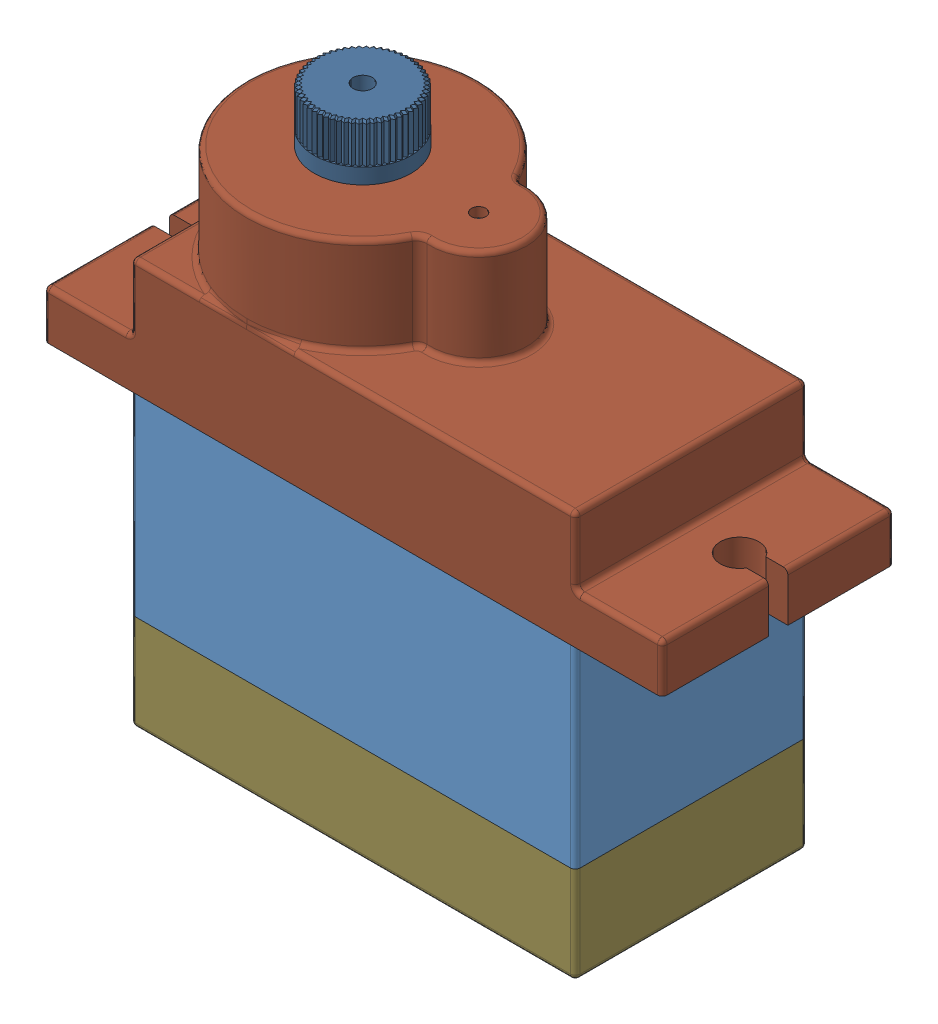
SolidWorks assembly SERVO 2, configuration Default. Lengths in mm.
Overall size (32 28.96 14.19).
25 component instances, 14 part files, 47 mates.
Components (placement in the parent):
- middle cover-1: middle cover [Default] at (8.87 8.8972 15.8774) size (23 11 12)
- shaft-1: shaft [Default] at (3.37 15.3972 15.8774) x (0 1 0) z (-0.985923 0 -0.167197) size (14.5 8.25 8.81)
- part 1-1: part 1 [Default] at (3.37 15.7972 15.8774) x (0 0 1) z (1 0 0) size (9.5 5.14 9.55)
- gear_sub1-1: gear_sub1 [Default] at (9.5 19.3472 15.8774) x (-0.853456 0 0.521165) z (-0.521165 0 -0.853456) size (10.24 10.65 10.25)
  - shaft^gear_sub1-1: shaft^gear_sub1 [Default] at origin size (1 10.65 1) (virtual)
  - spur gear_iso-2: spur gear_iso [ISO - Spur gear 0.25M 39T 20PA 1FW ---S39A75H50L0.8N] at (0 0.1 0) x (0 1 0) z (0 0 1) size (1 10.24 10.25)
  - spur gear_iso-5: spur gear_iso [ISO - Spur gear 0.25M 10T 20PA 1.75FW ---S10A75H50L1.0N] at (0 1.1 0) x (0 1 0) z (0 0 1) size (1.75 2.87 3)
- gear_sub2-1: gear_sub2 [Default] at (3.37 20.7972 15.8774) x (-0.834296 0 0.551317) z (-0.551317 0 -0.834296) size (10.24 2.75 10.25)
  - spur gear_iso-2: spur gear_iso [ISO - Spur gear 0.25M 39T 20PA 1FW ---S39A75H50L0.8N] at (0 0.1 0) x (0 1 0) z (0 0 1) size (1 10.24 10.25)
  - spur gear_iso-5: spur gear_iso [ISO - Spur gear 0.25M 10T 20PA 1.75FW ---S10A75H50L1.0N] at (0 1.1 0) x (0 1 0) z (0 0 1) size (1.75 2.87 3)
- pcb-1: pcb [Default] at (4.7516 11.69 15.8774) x (0.906308 0.422618 0) z (0 0 -1) size (10 2 9)
- wires1^SERVO 2-1: wires1^SERVO 2 [Default] at (8.87 8.8972 21.8774) (virtual)
- DC Motor as part-2: DC Motor as part [Default] at (20.0465 3.7393 19.3612) x (0 0 -1) z (0 1 0) size (8.04 6.55 11.14)
- Rotor scaled-1: Rotor scaled [Default] at (15.62 14.0372 15.8774) x (0.826635 0 -0.562739) z (0 1 0) size (5.2 5.12 15.2)
- spur gear_am-3: spur gear_am [Metric - Spur gear 0.25M 10T 20PA 2FW ---S10N75H50L0.8N] at (15.62 18.9472 15.8774) x (0 1 0) z (0.067436 0 0.997724) size (2 2.87 3)
- gear_sub3-2: gear_sub3 [Default] at (9.5126 21.8914 14.1824) x (-0.43734 0 -0.899296) z (0.899296 0 -0.43734) size (10.24 7 10.25)
  - spur gear_iso-2: spur gear_iso [ISO - Spur gear 0.25M 39T 20PA 1FW ---S39A75H50L0.8N] at (-1.5188 0.3058 -0.7526) x (0 1 0) z (0 0 1) size (1 10.24 10.25)
  - spur gear_iso-6: spur gear_iso [ISO - Spur gear 0.25M 10T 20PA 6FW ---S10A75H50L0.8N] at (-1.5188 1.3058 -0.7526) x (0 1 0) z (0 0 1) size (6 2.87 3)
- gear5-1: gear5 [Default] at (0.4816 -19.0533 15.951) x (0 -1 0) z (0.847043 0 0.531525) size (6.5 10.24 10.25)
- Part5-1: Part5 [Default] at (8.87 24.8972 15.8774) size (32 11 12.1)
- part 3 bottom-1: part 3 bottom [Default] at (8.87 3.8972 15.8774) size (23 5 12)
- Part6-1: Part6 [Default] at (-1.38 3.7472 11.1274) x (0 1 0) z (-0.44899 0 0.893537) size (20.01 2 2)
- Part6-2: Part6 [Default] at (-1.38 3.7472 20.6274) x (0 1 0) z (-0.272553 0 0.962141) size (20.01 2 2)
- Part6-4: Part6 [Default] at (19.12 3.7472 20.6274) x (0 1 0) z (-0.058733 0 0.998274) size (20.01 2 2)
- Part6-6: Part6 [Default] at (19.12 3.7472 11.1274) x (0 1 0) z (0.17693 0 0.984223) size (20.01 2 2)
Mates (geometry in assembly coordinates):
- Concentric1: concentric anti-aligned: cylinder of middle cover-1 through (3.37 8.8962 15.8774) axis (0 1 0) radius 5; cylinder of part 1-1 through (3.37 16.2972 15.8774) axis (0 -1 0) radius 4.75
- Concentric2: concentric aligned: cylinder of shaft-1 through (3.37 15.3972 15.8774) axis (0 -1 0) radius 0.6; cylinder of part 1-1 through (3.37 19.2972 15.8774) axis (0 -1 0) radius 4.5
- Tangent1: tangent: face of shaft-1; plane of part 1-1 through (4.8064 16.4472 14.6722) normal (0 1 0)
- Concentric3: concentric aligned: cylinder of shaft-1 through (3.37 15.3972 15.8774) axis (0 -1 0) radius 0.5; cylinder of gear_sub2-1/spur gear_iso-5 through (3.37 71.8973 15.8774) axis (0 -1 0) radius 0.5
- Coincident6: coincident anti-aligned: plane of shaft-1 through (3.4536 20.8972 15.3844) normal (0 1 0); plane of gear_sub2-1/spur gear_iso-2 through (3.37 20.8972 15.8774) normal (0 -1 0)
- Concentric4: concentric aligned: cylinder of middle cover-1 through (9.5 19.4472 15.8774) axis (0 -1 0) radius 0.5; cylinder of gear_sub1-1/shaft^gear_sub1-1 through (9.5 18.6972 15.8774) axis (0 -1 0) radius 0.5
- Width1: width anti-aligned: plane of pcb-1 through (9.6001 13.1234 20.3774) normal (0 0 1); plane of pcb-1 through (9.6001 13.1234 11.3774) normal (0 0 -1); plane of middle cover-1 through (20.37 18.8972 20.8774) normal (0 0 -1); plane of middle cover-1 through (20.37 18.8972 10.8774) normal (0 0 1)
- Coincident9: coincident: plane of middle cover-1 through (8.87 8.8972 15.8774) normal (0 -1 0); line of pcb-1 through (0.537 8.8972 20.3774) axis (0 0 -1)
- Angle1: planar angle = 0.436332 rad aligned: plane of pcb-1 through (5.0685 11.0103 15.8774) normal (0.422618 -0.906308 0); plane of middle cover-1 through (8.87 8.8972 15.8774) normal (0 -1 0)
- Tangent2: tangent: cylinder of middle cover-1 through (-1.38 18.8972 20.6274) axis (0 -1 0) radius 1.6; line of pcb-1 through (0.22 9.5769 20.3774) axis (0 0 -1)
- InPlace1: in place: plane of middle cover-1 through (20.37 18.8972 21.8774) normal (0 0 1); plane of ? through (0 0 21.8774) normal (0 0 1); moOrthogonalPlaneRef_w of middle cover-1 through (20.37 18.8972 21.8774) normal (0 0 1); plane of ? through (0 0 21.8774) normal (0 1 0); plane of middle cover-1 through (20.37 18.8972 21.8774) normal (0 0 1); plane of ? through (0 0 21.8774) normal (1 0 0); plane of middle cover-1 through (20.37 18.8972 21.8774) normal (0 0 1); unknown of wires1^SERVO 2-1
- Coincident11: coincident aligned: plane of middle cover-1; plane of wires1^SERVO 2-1
- Coincident12: coincident aligned: moOrthogonalPlaneRef_w of middle cover-1 through (8.87 8.8972 21.8774) normal (0 1 0); plane of wires1^SERVO 2-1 through (8.87 8.8972 21.8774) normal (0 1 0)
- Coincident13: coincident anti-aligned: moOrthogonalPlaneRef_w of middle cover-1 through (8.87 8.8972 21.8774) normal (-1 0 0); plane of wires1^SERVO 2-1 through (8.87 8.8972 21.8774) normal (1 0 0)
- Concentric5: concentric aligned: cylinder of middle cover-1 through (15.62 8.8962 15.8774) axis (0 1 0) radius 1.55; cylinder of DC Motor as part-2 through (15.62 17.7472 15.8774) axis (0 1 0) radius 0.4
- Parallel5: parallel anti-aligned: plane of middle cover-1 through (12.22 12.8972 19.2524) normal (1 0 0); plane of DC Motor as part-2 through (12.62 17.8972 18.5231) normal (-1 0 0)
- Coincident11: coincident anti-aligned: plane of middle cover-1 through (8.87 17.8972 15.8774) normal (0 -1 0); plane of DC Motor as part-2 through (15.62 17.8972 15.8774) normal (0 1 0)
- Coincident12: coincident anti-aligned: circle of DC Motor as part-2; cylinder of Rotor scaled-1 through (15.62 21.6372 15.8774) axis (0 -1 0) radius 0.4
- Coincident13: coincident aligned: plane of DC Motor as part-2 through (14.486 9.2572 14.5254) normal (0 -1 0); plane of Rotor scaled-1 through (15.62 9.2572 15.8774) normal (0 -1 0)
- Coincident15: coincident anti-aligned: plane of middle cover-1 through (8.87 15.2972 15.8774) normal (0 1 0); plane of part 1-1 through (3.37 15.2972 15.8774) normal (0 -1 0)
- Parallel7: parallel aligned: plane of middle cover-1 through (4.62 14.7972 10.8774) normal (1 0 0); plane of part 1-1 through (4.37 15.2972 15.8774) normal (1 0 0)
- Concentric7: concentric aligned: cylinder of Rotor scaled-1 through (15.62 21.6372 15.8774) axis (0 -1 0) radius 0.4; cylinder of spur gear_am-3 through (15.62 68.9473 15.8774) axis (0 -1 0) radius 0.4
- Width2: width aligned: plane of gear_sub1-1/spur gear_iso-2 through (9.5 20.4472 15.8774) normal (0 1 0); plane of gear_sub1-1/spur gear_iso-2 through (9.5 19.4472 15.8774) normal (0 -1 0); plane of spur gear_am-3 through (15.62 20.9472 15.8774) normal (0 1 0); plane of spur gear_am-3 through (15.62 18.9472 15.8774) normal (0 -1 0)
- Lock1: lock: unknown of Rotor scaled-1; unknown of spur gear_am-3
- Concentric8: concentric anti-aligned: cylinder of gear_sub1-1/shaft^gear_sub1-1 through (9.5 18.6972 15.8774) axis (0 1 0) radius 0.5; cylinder of gear_sub3-2/spur gear_iso-6 through (9.5 73.1973 15.8774) axis (0 -1 0) radius 0.4
- Coincident16: coincident anti-aligned: plane of gear_sub1-1/spur gear_iso-5 through (9.5 22.1972 15.8774) normal (0 1 0); plane of gear_sub3-2/spur gear_iso-2 through (9.5 22.1972 15.8774) normal (0 -1 0)
- Concentric9: concentric anti-aligned: cylinder of shaft-1 through (3.37 15.3972 15.8774) axis (0 -1 0) radius 0.6; cylinder of gear5-1 through (3.37 -20.8028 15.8774) axis (0 1 0) radius 0.5
- GearMate5: gear = 39 : 10 mm: cylinder of spur gear_am-3 through (15.62 20.9472 15.8774) axis (0 -1 0) radius 0.9365; cylinder of gear_sub1-1/spur gear_iso-2 through (9.5 20.4472 15.8774) axis (0 -1 0) radius 4.5615
- GearMate6: gear = 39 : 10 mm: cylinder of gear_sub1-1/spur gear_iso-5 through (9.5 22.1972 15.8774) axis (0 -1 0) radius 0.9365; cylinder of gear_sub2-1/spur gear_iso-2 through (3.37 21.8972 15.8774) axis (0 -1 0) radius 4.5615
- GearMate7: gear = 39 : 10 mm: cylinder of gear_sub2-1/spur gear_iso-5 through (3.37 23.6472 15.8774) axis (0 -1 0) radius 0.9365; cylinder of gear_sub3-2/spur gear_iso-2 through (9.5 23.1972 15.8774) axis (0 -1 0) radius 4.5615
- GearMate8: gear = 39 : 10 mm: cylinder of gear_sub3-2/spur gear_iso-6 through (9.5 29.1972 15.8774) axis (0 -1 0) radius 0.9365; cylinder of gear5-1 through (3.37 26.1972 15.8774) axis (0 1 0) radius 4.5615
- Coincident17: coincident aligned: plane of gear_sub3-2/spur gear_iso-6 through (9.5 29.1972 15.8774) normal (0 1 0); plane of gear5-1 through (3.37 29.1972 15.8774) normal (0 1 0)
- Lock3: lock: unknown of shaft-1; unknown of gear5-1
- Concentric11: concentric anti-aligned: cylinder of middle cover-1 through (-1.38 19.8972 20.6274) axis (0 -1 0) radius 1; cylinder of Part5-1 through (-1.38 18.8972 20.6274) axis (0 1 0) radius 1
- Concentric12: concentric anti-aligned: cylinder of middle cover-1 through (19.12 19.8972 11.1274) axis (0 -1 0) radius 1; cylinder of Part5-1 through (19.12 18.8972 11.1274) axis (0 1 0) radius 1
- Coincident18: coincident anti-aligned: plane of middle cover-1 through (8.87 18.8972 15.8774) normal (0 1 0); plane of Part5-1 through (8.87 18.8972 15.8774) normal (0 -1 0)
- Coincident19: coincident anti-aligned: plane of middle cover-1 through (8.87 8.8972 15.8774) normal (0 -1 0); plane of part 3 bottom-1 through (8.87 8.8972 15.8774) normal (0 1 0)
- Concentric13: concentric aligned: cylinder of middle cover-1 through (-1.38 18.8972 20.6274) axis (0 -1 0) radius 0.6; cylinder of part 3 bottom-1 through (-1.38 8.8972 20.6274) axis (0 -1 0) radius 1
- Concentric14: concentric aligned: cylinder of middle cover-1 through (19.12 18.8972 20.6274) axis (0 -1 0) radius 0.6; cylinder of part 3 bottom-1 through (19.12 8.8972 20.6274) axis (0 -1 0) radius 1
- Concentric16: concentric aligned: cylinder of part 3 bottom-1 through (-1.38 7.2472 11.1274) axis (0 -1 0) radius 0.6; cylinder of Part6-1 through (-1.38 3.7472 11.1274) axis (0 -1 0) radius 0.5
- Coincident22: coincident anti-aligned: plane of part 3 bottom-1 through (-1.38 4.7472 11.1274) normal (0 -1 0); plane of Part6-1 through (-1.8267 4.7472 10.9029) normal (0 1 0)
- Concentric17: concentric aligned: cylinder of part 3 bottom-1 through (-1.38 7.2472 20.6274) axis (0 -1 0) radius 0.6; cylinder of Part6-2 through (-1.38 3.7472 20.6274) axis (0 -1 0) radius 0.5
- Coincident23: coincident anti-aligned: plane of part 3 bottom-1 through (-1.38 4.7472 20.6274) normal (0 -1 0); plane of Part6-2 through (-1.861 4.7472 20.4911) normal (0 1 0)
- Concentric18: concentric aligned: cylinder of part 3 bottom-1 through (19.12 7.2472 20.6274) axis (0 -1 0) radius 0.6; cylinder of Part6-4 through (19.12 3.7472 20.6274) axis (0 -1 0) radius 0.5
- Coincident24: coincident anti-aligned: plane of part 3 bottom-1 through (19.12 4.7472 20.6274) normal (0 -1 0); plane of Part6-4 through (18.6209 4.7472 20.598) normal (0 1 0)
- Concentric19: concentric aligned: cylinder of part 3 bottom-1 through (19.12 7.2472 11.1274) axis (0 -1 0) radius 0.6; cylinder of Part6-6 through (19.12 3.7472 11.1274) axis (0 -1 0) radius 0.5
- Coincident25: coincident anti-aligned: plane of part 3 bottom-1 through (19.12 4.7472 11.1274) normal (0 -1 0); plane of Part6-6 through (18.6279 4.7472 11.2158) normal (0 1 0)
